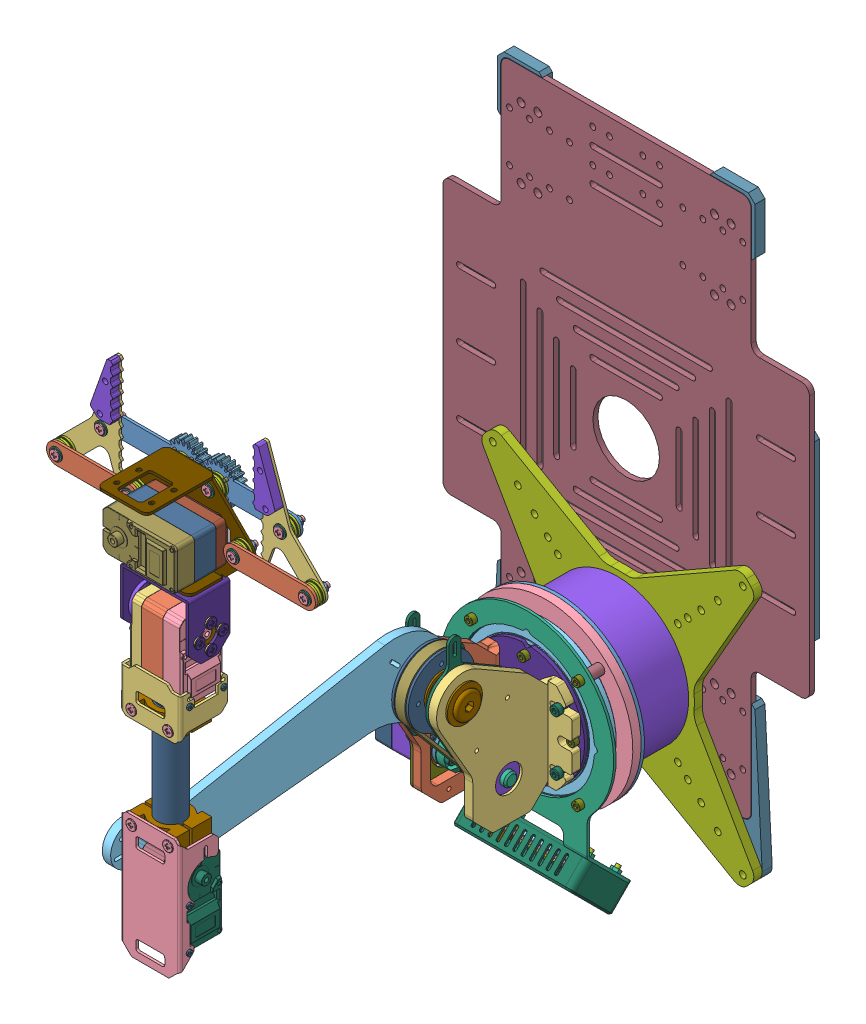
SolidWorks assembly RoArm-M1 STEP, configuration Default. Lengths in mm. (continued)
Components (placement in the parent): (continued)
- RoArm-M1 STEP(2)^RoArm-M1 STEP-1: RoArm-M1 STEP(2)^RoArm-M1 STEP [Default] at origin size (176.32 372.07 316.7) (virtual) (continued)
  - Servo Driver with ESP32^RoArm-M1 STEP(2)_RoArm-M1 STEP-1: Servo Driver with ESP32^RoArm-M1 STEP(2)_RoArm-M1 STEP [Default] at (-32.5 -89.0448 39.0323) x (1 0 0) z (0 -0.707107 0.707107) size (65.89 30.51 11.2) (virtual) (continued)
    - Servo Driver with ESP32-0^Servo Driver with ESP32_RoArm-M1 STEP(2)_RoArm-M1 STEP-1: Servo Driver with ESP32-0^Servo Driver with ESP32_RoArm-M1 STEP(2)_RoArm-M1 STEP [Default] at origin size (11 5 5.7) (virtual)
    - Servo Driver with ESP32-1^Servo Driver with ESP32_RoArm-M1 STEP(2)_RoArm-M1 STEP-1: Servo Driver with ESP32-1^Servo Driver with ESP32_RoArm-M1 STEP(2)_RoArm-M1 STEP [Default] at origin size (0.71 0.71 7.5) (virtual)
    - Servo Driver with ESP32-2^Servo Driver with ESP32_RoArm-M1 STEP(2)_RoArm-M1 STEP-1: Servo Driver with ESP32-2^Servo Driver with ESP32_RoArm-M1 STEP(2)_RoArm-M1 STEP [Default] at origin size (0.71 0.71 7.5) (virtual)
    - Servo Driver with ESP32-3^Servo Driver with ESP32_RoArm-M1 STEP(2)_RoArm-M1 STEP-1: Servo Driver with ESP32-3^Servo Driver with ESP32_RoArm-M1 STEP(2)_RoArm-M1 STEP [Default] at origin size (0.71 0.71 7.5) (virtual)
    - Servo Driver with ESP32-4^Servo Driver with ESP32_RoArm-M1 STEP(2)_RoArm-M1 STEP-1: Servo Driver with ESP32-4^Servo Driver with ESP32_RoArm-M1 STEP(2)_RoArm-M1 STEP [Default] at origin size (11 5 8.5) (virtual)
    - Servo Driver with ESP32-5^Servo Driver with ESP32_RoArm-M1 STEP(2)_RoArm-M1 STEP-1: Servo Driver with ESP32-5^Servo Driver with ESP32_RoArm-M1 STEP(2)_RoArm-M1 STEP [Default] at origin size (0.7 0.7 7.5) (virtual)
    - Servo Driver with ESP32-6^Servo Driver with ESP32_RoArm-M1 STEP(2)_RoArm-M1 STEP-1: Servo Driver with ESP32-6^Servo Driver with ESP32_RoArm-M1 STEP(2)_RoArm-M1 STEP [Default] at origin size (0.71 0.71 7.5) (virtual)
  - 碳管前固定^RoArm-M1 STEP(2)_RoArm-M1 STEP-1: 碳管前固定^RoArm-M1 STEP(2)_RoArm-M1 STEP [Default] at (66.1341 -832.2469 298.6056) x (0 -1 0) z (0 0 1) size (28.35 36.11 28.3) (virtual)
  - 碳管后固定^RoArm-M1 STEP(2)_RoArm-M1 STEP-1: 碳管后固定^RoArm-M1 STEP(2)_RoArm-M1 STEP [Default] at (-73.8484 -939.3227 298.6056) x (0 -1 0) z (0 0 1) size (73.69 35.71 23.05) (virtual)
  - 机械臂大臂^RoArm-M1 STEP(2)_RoArm-M1 STEP-1: 机械臂大臂^RoArm-M1 STEP(2)_RoArm-M1 STEP [Default] at (-4.9615 -12.5543 693.461) x (0 0 1) z (-1 0 0) size (207.69 52.86 5) (virtual)
  - 中心外侧PCB支架^RoArm-M1 STEP(2)_RoArm-M1 STEP-1: 中心外侧PCB支架^RoArm-M1 STEP(2)_RoArm-M1 STEP [Default] at (18.4653 1675.6917 58) x (0 -1 0) z (0 0 1) size (138.15 104 27.96) (virtual)
  - X型底座^RoArm-M1 STEP(2)_RoArm-M1 STEP-1: X型底座^RoArm-M1 STEP(2)_RoArm-M1 STEP [Default] at (2038.816 -62.8687 0) x (-1 0 0) z (0 0 1) size (163.25 163.25 5) (virtual)
  - 厚铝管^RoArm-M1 STEP(2)_RoArm-M1 STEP-1: 厚铝管^RoArm-M1 STEP(2)_RoArm-M1 STEP [Default] at (0 0 5) x (-1 0 0) z (0 0 1) size (85 85 36) (virtual)
  - LEG-HOLDER^RoArm-M1 STEP(2)_RoArm-M1 STEP-1: LEG-HOLDER^RoArm-M1 STEP(2)_RoArm-M1 STEP [Default] at (14.5485 57.813 287.8556) x (-1 0 0) z (0 1 0) size (28 21.5 10.1) (virtual)
  - LEG-HOLDER^RoArm-M1 STEP(2)_RoArm-M1 STEP-2: LEG-HOLDER^RoArm-M1 STEP(2)_RoArm-M1 STEP [Default] at (14.5485 117.713 287.8556) x (-1 0 0) z (0 1 0) size (28 21.5 10.1) (virtual)
  - 70mm碳纤维管材^RoArm-M1 STEP(2)_RoArm-M1 STEP-1: 70mm碳纤维管材^RoArm-M1 STEP(2)_RoArm-M1 STEP [Default] at (-267.2094 57.813 273.529) x (-1 0 0) z (0 1 0) size (16 16 70) (virtual)
  - 圆形隔离柱 M3_35^RoArm-M1 STEP(2)_RoArm-M1 STEP-1: 圆形隔离柱 M3_35^RoArm-M1 STEP(2)_RoArm-M1 STEP [Default] at (-24.3952 24.3952 5) x (-1 0 0) z (0 0 1) size (6 6 35) (virtual)
  - 圆形隔离柱 M3_35^RoArm-M1 STEP(2)_RoArm-M1 STEP-2: 圆形隔离柱 M3_35^RoArm-M1 STEP(2)_RoArm-M1 STEP [Default] at (-24.3952 -24.3952 5) x (-1 0 0) z (0 0 1) size (6 6 35) (virtual)
  - 圆形隔离柱 M3_35^RoArm-M1 STEP(2)_RoArm-M1 STEP-3: 圆形隔离柱 M3_35^RoArm-M1 STEP(2)_RoArm-M1 STEP [Default] at (24.3952 -24.3952 5) x (-1 0 0) z (0 0 1) size (6 6 35) (virtual)
  - 圆形隔离柱 M3_35^RoArm-M1 STEP(2)_RoArm-M1 STEP-4: 圆形隔离柱 M3_35^RoArm-M1 STEP(2)_RoArm-M1 STEP [Default] at (24.3952 24.3952 5) x (-1 0 0) z (0 0 1) size (6 6 35) (virtual)
  - 黑色金属沉头螺丝 KM3_10^RoArm-M1 STEP(2)_RoArm-M1 STEP-1: 黑色金属沉头螺丝 KM3_10^RoArm-M1 STEP(2)_RoArm-M1 STEP [Default] at (24.3952 -24.3952 12) x (-1 0 0) z (0 0 -1) size (5.2 5.2 6) (virtual)
  - 黑色金属沉头螺丝 KM3_10^RoArm-M1 STEP(2)_RoArm-M1 STEP-2: 黑色金属沉头螺丝 KM3_10^RoArm-M1 STEP(2)_RoArm-M1 STEP [Default] at (24.3952 24.3952 12) x (-1 0 0) z (0 0 -1) size (5.2 5.2 6) (virtual)
  - 黑色金属沉头螺丝 KM3_10^RoArm-M1 STEP(2)_RoArm-M1 STEP-3: 黑色金属沉头螺丝 KM3_10^RoArm-M1 STEP(2)_RoArm-M1 STEP [Default] at (-24.3952 -24.3952 12) x (-1 0 0) z (0 0 -1) size (5.2 5.2 6) (virtual)
  - 黑色金属沉头螺丝 KM3_10^RoArm-M1 STEP(2)_RoArm-M1 STEP-4: 黑色金属沉头螺丝 KM3_10^RoArm-M1 STEP(2)_RoArm-M1 STEP [Default] at (-24.3952 24.3952 12) x (-1 0 0) z (0 0 -1) size (5.2 5.2 6) (virtual)
  - 圆形隔离柱 M3_10^RoArm-M1 STEP(2)_RoArm-M1 STEP-1: 圆形隔离柱 M3_10^RoArm-M1 STEP(2)_RoArm-M1 STEP [Default] at (32.1734 -32.1734 48) x (-1 0 0) z (0 0 1) size (6 6 10) (virtual)
  - 圆形隔离柱 M3_10^RoArm-M1 STEP(2)_RoArm-M1 STEP-2: 圆形隔离柱 M3_10^RoArm-M1 STEP(2)_RoArm-M1 STEP [Default] at (32.1734 32.1734 48) x (-1 0 0) z (0 0 1) size (6 6 10) (virtual)
  - 圆形隔离柱 M3_10^RoArm-M1 STEP(2)_RoArm-M1 STEP-3: 圆形隔离柱 M3_10^RoArm-M1 STEP(2)_RoArm-M1 STEP [Default] at (-32.1734 32.1734 48) x (-1 0 0) z (0 0 1) size (6 6 10) (virtual)
  - 圆形隔离柱 M3_10^RoArm-M1 STEP(2)_RoArm-M1 STEP-4: 圆形隔离柱 M3_10^RoArm-M1 STEP(2)_RoArm-M1 STEP [Default] at (-32.1734 -32.1734 48) x (-1 0 0) z (0 0 1) size (6 6 10) (virtual)
  - 黑色金属圆头尖尾自攻螺丝 PA2_5^RoArm-M1 STEP(2)_RoArm-M1 STEP-1: 黑色金属圆头尖尾自攻螺丝 PA2_5^RoArm-M1 STEP(2)_RoArm-M1 STEP [Default] at (8.3 -10.25 43) x (-1 0 0) z (0 0 1) size (3.35 3.35 6.15) (virtual)
  - 黑色金属圆头尖尾自攻螺丝 PA2_5^RoArm-M1 STEP(2)_RoArm-M1 STEP-2: 黑色金属圆头尖尾自攻螺丝 PA2_5^RoArm-M1 STEP(2)_RoArm-M1 STEP [Default] at (29 -10.25 43) x (-1 0 0) z (0 0 1) size (3.35 3.35 6.15) (virtual)
  - 黑色金属圆头尖尾自攻螺丝 PA2_5^RoArm-M1 STEP(2)_RoArm-M1 STEP-3: 黑色金属圆头尖尾自攻螺丝 PA2_5^RoArm-M1 STEP(2)_RoArm-M1 STEP [Default] at (8.3 10.25 43) x (-1 0 0) z (0 0 1) size (3.35 3.35 6.15) (virtual)
  - 黑色金属圆头尖尾自攻螺丝 PA2_5^RoArm-M1 STEP(2)_RoArm-M1 STEP-4: 黑色金属圆头尖尾自攻螺丝 PA2_5^RoArm-M1 STEP(2)_RoArm-M1 STEP [Default] at (29 10.25 43) x (-1 0 0) z (0 0 1) size (3.35 3.35 6.15) (virtual)
  - 黑色金属圆头尖尾自攻螺丝 PA2_5^RoArm-M1 STEP(2)_RoArm-M1 STEP-5: 黑色金属圆头尖尾自攻螺丝 PA2_5^RoArm-M1 STEP(2)_RoArm-M1 STEP [Default] at (-17.9615 -3.5824 98.625) x (0 0 1) z (1 0 0) size (3.35 3.35 6.15) (virtual)
  - 黑色金属圆头尖尾自攻螺丝 PA2_5^RoArm-M1 STEP(2)_RoArm-M1 STEP-6: 黑色金属圆头尖尾自攻螺丝 PA2_5^RoArm-M1 STEP(2)_RoArm-M1 STEP [Default] at (-17.9615 17.1176 98.625) x (0 0 1) z (1 0 0) size (3.35 3.35 6.15) (virtual)
  - 黑色金属圆头尖尾自攻螺丝 PA2_5^RoArm-M1 STEP(2)_RoArm-M1 STEP-7: 黑色金属圆头尖尾自攻螺丝 PA2_5^RoArm-M1 STEP(2)_RoArm-M1 STEP [Default] at (-17.9615 17.1176 78.125) x (0 0 1) z (1 0 0) size (3.35 3.35 6.15) (virtual)
  - 黑色金属圆头尖尾自攻螺丝 PA2_5^RoArm-M1 STEP(2)_RoArm-M1 STEP-8: 黑色金属圆头尖尾自攻螺丝 PA2_5^RoArm-M1 STEP(2)_RoArm-M1 STEP [Default] at (-17.9615 -3.5824 78.125) x (0 0 1) z (1 0 0) size (3.35 3.35 6.15) (virtual)
  - 黑色金属圆头尖尾自攻螺丝 PA2_5^RoArm-M1 STEP(2)_RoArm-M1 STEP-9: 黑色金属圆头尖尾自攻螺丝 PA2_5^RoArm-M1 STEP(2)_RoArm-M1 STEP [Default] at (32.3585 32.7513 294.848) x (0 0 1) z (1 0 0) size (3.35 3.35 6.15) (virtual)
  - 黑色金属圆头尖尾自攻螺丝 PA2_5^RoArm-M1 STEP(2)_RoArm-M1 STEP-10: 黑色金属圆头尖尾自攻螺丝 PA2_5^RoArm-M1 STEP(2)_RoArm-M1 STEP [Default] at (32.3585 8.3013 294.848) x (0 0 1) z (1 0 0) size (3.35 3.35 6.15) (virtual)
  - 黑色金属圆头尖尾自攻螺丝 PA2_5^RoArm-M1 STEP(2)_RoArm-M1 STEP-11: 黑色金属圆头尖尾自攻螺丝 PA2_5^RoArm-M1 STEP(2)_RoArm-M1 STEP [Default] at (-1.7615 12.0513 294.848) x (0 0 -1) z (-1 0 0) size (3.35 3.35 6.15) (virtual)
  - 黑色金属圆头尖尾自攻螺丝 PA2_5^RoArm-M1 STEP(2)_RoArm-M1 STEP-12: 黑色金属圆头尖尾自攻螺丝 PA2_5^RoArm-M1 STEP(2)_RoArm-M1 STEP [Default] at (-1.7615 32.7513 294.848) x (0 0 -1) z (-1 0 0) size (3.35 3.35 6.15) (virtual)
  - 黑色金属圆头尖尾自攻螺丝 PA2_5^RoArm-M1 STEP(2)_RoArm-M1 STEP-13: 黑色金属圆头尖尾自攻螺丝 PA2_5^RoArm-M1 STEP(2)_RoArm-M1 STEP [Default] at (-3.4615 139.9747 294.848) x (0 0 -1) z (-1 0 0) size (3.35 3.35 6.15) (virtual)
  - 黑色金属圆头尖尾自攻螺丝 PA2_5^RoArm-M1 STEP(2)_RoArm-M1 STEP-14: 黑色金属圆头尖尾自攻螺丝 PA2_5^RoArm-M1 STEP(2)_RoArm-M1 STEP [Default] at (-3.4615 139.9747 274.348) x (0 0 -1) z (-1 0 0) size (3.35 3.35 6.15) (virtual)
  - 黑色金属圆头尖尾自攻螺丝 PA2_5^RoArm-M1 STEP(2)_RoArm-M1 STEP-15: 黑色金属圆头尖尾自攻螺丝 PA2_5^RoArm-M1 STEP(2)_RoArm-M1 STEP [Default] at (32.5585 136.2247 294.848) x (0 0 1) z (1 0 0) size (3.35 3.35 6.15) (virtual)
  - 黑色金属圆头尖尾自攻螺丝 PA2_5^RoArm-M1 STEP(2)_RoArm-M1 STEP-16: 黑色金属圆头尖尾自攻螺丝 PA2_5^RoArm-M1 STEP(2)_RoArm-M1 STEP [Default] at (32.5585 136.2247 274.348) x (0 0 1) z (1 0 0) size (3.35 3.35 6.15) (virtual)
  - 黑色金属圆头尖尾自攻螺丝 PA2_5^RoArm-M1 STEP(2)_RoArm-M1 STEP-17: 黑色金属圆头尖尾自攻螺丝 PA2_5^RoArm-M1 STEP(2)_RoArm-M1 STEP [Default] at (30.4885 203.7559 273.6404) x (0 1 0) z (0 0 -1) size (3.35 3.35 6.15) (virtual)
  - 黑色金属圆头尖尾自攻螺丝 PA2_5^RoArm-M1 STEP(2)_RoArm-M1 STEP-18: 黑色金属圆头尖尾自攻螺丝 PA2_5^RoArm-M1 STEP(2)_RoArm-M1 STEP [Default] at (9.7885 203.7559 273.6404) x (0 1 0) z (0 0 -1) size (3.35 3.35 6.15) (virtual)
  - 黑色金属圆头尖尾自攻螺丝 PA2_5^RoArm-M1 STEP(2)_RoArm-M1 STEP-19: 黑色金属圆头尖尾自攻螺丝 PA2_5^RoArm-M1 STEP(2)_RoArm-M1 STEP [Default] at (30.4885 224.2559 273.6404) x (0 1 0) z (0 0 -1) size (3.35 3.35 6.15) (virtual)
  - 黑色金属圆头尖尾自攻螺丝 PA2_5^RoArm-M1 STEP(2)_RoArm-M1 STEP-20: 黑色金属圆头尖尾自攻螺丝 PA2_5^RoArm-M1 STEP(2)_RoArm-M1 STEP [Default] at (9.7885 224.2559 273.6404) x (0 1 0) z (0 0 -1) size (3.35 3.35 6.15) (virtual)
  - 黑色金属杯头内六角螺丝 M3_8^RoArm-M1 STEP(2)_RoArm-M1 STEP-1: 黑色金属杯头内六角螺丝 M3_8^RoArm-M1 STEP(2)_RoArm-M1 STEP [Default] at (-11.2615 -11.8824 95.375) x (0 0 1) z (1 0 0) size (5.5 5.5 11.1) (virtual)
  - 黑色金属杯头内六角螺丝 M3_8^RoArm-M1 STEP(2)_RoArm-M1 STEP-2: 黑色金属杯头内六角螺丝 M3_8^RoArm-M1 STEP(2)_RoArm-M1 STEP [Default] at (-16.2615 -11.8824 88.375) x (0 0 1) z (1 0 0) size (5.5 5.5 11.1) (virtual)
  - 黑色金属杯头内六角螺丝 M3_8^RoArm-M1 STEP(2)_RoArm-M1 STEP-3: 黑色金属杯头内六角螺丝 M3_8^RoArm-M1 STEP(2)_RoArm-M1 STEP [Default] at (-11.2615 -18.8824 88.375) x (0 0 1) z (1 0 0) size (5.5 5.5 11.1) (virtual)
  - 黑色金属杯头内六角螺丝 M3_8^RoArm-M1 STEP(2)_RoArm-M1 STEP-4: 黑色金属杯头内六角螺丝 M3_8^RoArm-M1 STEP(2)_RoArm-M1 STEP [Default] at (-11.2615 -4.8824 88.375) x (0 0 1) z (1 0 0) size (5.5 5.5 11.1) (virtual)
  - 黑色金属杯头内六角螺丝 M3_8^RoArm-M1 STEP(2)_RoArm-M1 STEP-5: 黑色金属杯头内六角螺丝 M3_8^RoArm-M1 STEP(2)_RoArm-M1 STEP [Default] at (-11.2615 -11.8824 81.375) x (0 0 1) z (1 0 0) size (5.5 5.5 11.1) (virtual)
  - 黑色金属杯头内六角螺丝 M3_8^RoArm-M1 STEP(2)_RoArm-M1 STEP-6: 黑色金属杯头内六角螺丝 M3_8^RoArm-M1 STEP(2)_RoArm-M1 STEP [Default] at (24.9 -16.5003 65) x (-1 0 0) z (0 0 1) size (5.5 5.5 11.1) (virtual)
  - 黑色金属杯头内六角螺丝 M3_8^RoArm-M1 STEP(2)_RoArm-M1 STEP-7: 黑色金属杯头内六角螺丝 M3_8^RoArm-M1 STEP(2)_RoArm-M1 STEP [Default] at (24.9 16.5003 65) x (-1 0 0) z (0 0 1) size (5.5 5.5 11.1) (virtual)
  - 黑色金属杯头内六角螺丝 M3_8^RoArm-M1 STEP(2)_RoArm-M1 STEP-8: 黑色金属杯头内六角螺丝 M3_8^RoArm-M1 STEP(2)_RoArm-M1 STEP [Default] at (-24.9 -16.5003 65) x (-1 0 0) z (0 0 1) size (5.5 5.5 11.1) (virtual)
  - 黑色金属杯头内六角螺丝 M3_8^RoArm-M1 STEP(2)_RoArm-M1 STEP-9: 黑色金属杯头内六角螺丝 M3_8^RoArm-M1 STEP(2)_RoArm-M1 STEP [Default] at (-24.9 16.5003 65) x (-1 0 0) z (0 0 1) size (5.5 5.5 11.1) (virtual)
  - 银色金属杯头内六角螺丝 M3_6^RoArm-M1 STEP(2)_RoArm-M1 STEP-1: 银色金属杯头内六角螺丝 M3_6^RoArm-M1 STEP(2)_RoArm-M1 STEP [Default] at (-32.1734 32.1734 59.5) x (-1 0 0) z (0 0 1) size (5 5 9.1) (virtual)
  - 银色金属杯头内六角螺丝 M3_6^RoArm-M1 STEP(2)_RoArm-M1 STEP-2: 银色金属杯头内六角螺丝 M3_6^RoArm-M1 STEP(2)_RoArm-M1 STEP [Default] at (-32.1734 -32.1734 59.5) x (-1 0 0) z (0 0 1) size (5 5 9.1) (virtual)
  - 银色金属杯头内六角螺丝 M3_6^RoArm-M1 STEP(2)_RoArm-M1 STEP-3: 银色金属杯头内六角螺丝 M3_6^RoArm-M1 STEP(2)_RoArm-M1 STEP [Default] at (32.1734 32.1734 59.5) x (-1 0 0) z (0 0 1) size (5 5 9.1) (virtual)
  - 银色金属杯头内六角螺丝 M3_6^RoArm-M1 STEP(2)_RoArm-M1 STEP-4: 银色金属杯头内六角螺丝 M3_6^RoArm-M1 STEP(2)_RoArm-M1 STEP [Default] at (32.1734 -32.1734 59.5) x (-1 0 0) z (0 0 1) size (5 5 9.1) (virtual)
  - 圆形隔离柱 M3_10^RoArm-M1 STEP(2)_RoArm-M1 STEP-5: 圆形隔离柱 M3_10^RoArm-M1 STEP(2)_RoArm-M1 STEP [Default] at (29.5 0 48) x (-1 0 0) z (0 0 1) size (6 6 10) (virtual)
  - 圆形隔离柱 M3_10^RoArm-M1 STEP(2)_RoArm-M1 STEP-6: 圆形隔离柱 M3_10^RoArm-M1 STEP(2)_RoArm-M1 STEP [Default] at (0 29.5 48) x (-1 0 0) z (0 0 1) size (6 6 10) (virtual)
  - 圆形隔离柱 M3_10^RoArm-M1 STEP(2)_RoArm-M1 STEP-7: 圆形隔离柱 M3_10^RoArm-M1 STEP(2)_RoArm-M1 STEP [Default] at (-29.5 0 48) x (-1 0 0) z (0 0 1) size (6 6 10) (virtual)
  - 圆形隔离柱 M3_10^RoArm-M1 STEP(2)_RoArm-M1 STEP-8: 圆形隔离柱 M3_10^RoArm-M1 STEP(2)_RoArm-M1 STEP [Default] at (0 -29.5 48) x (-1 0 0) z (0 0 1) size (6 6 10) (virtual)
  - 银色金属杯头内六角螺丝 M3_6^RoArm-M1 STEP(2)_RoArm-M1 STEP-5: 银色金属杯头内六角螺丝 M3_6^RoArm-M1 STEP(2)_RoArm-M1 STEP [Default] at (29.5 0 60) x (-1 0 0) z (0 0 1) size (5 5 9.1) (virtual)
  - 银色金属杯头内六角螺丝 M3_6^RoArm-M1 STEP(2)_RoArm-M1 STEP-6: 银色金属杯头内六角螺丝 M3_6^RoArm-M1 STEP(2)_RoArm-M1 STEP [Default] at (0 29.5 60) x (-1 0 0) z (0 0 1) size (5 5 9.1) (virtual)
  - 银色金属杯头内六角螺丝 M3_6^RoArm-M1 STEP(2)_RoArm-M1 STEP-7: 银色金属杯头内六角螺丝 M3_6^RoArm-M1 STEP(2)_RoArm-M1 STEP [Default] at (-29.5 0 60) x (-1 0 0) z (0 0 1) size (5 5 9.1) (virtual)
  - 银色金属杯头内六角螺丝 M3_6^RoArm-M1 STEP(2)_RoArm-M1 STEP-8: 银色金属杯头内六角螺丝 M3_6^RoArm-M1 STEP(2)_RoArm-M1 STEP [Default] at (0 -29.5 60) x (-1 0 0) z (0 0 1) size (5 5 9.1) (virtual)
  - 黑色金属扁平头螺丝 CM3_6_6^RoArm-M1 STEP(2)_RoArm-M1 STEP-1: 黑色金属扁平头螺丝 CM3_6_6^RoArm-M1 STEP(2)_RoArm-M1 STEP [Default] at (24.3952 24.3952 43) x (-1 0 0) z (0 0 1) size (6 6 6.8) (virtual)
  - 黑色金属扁平头螺丝 CM3_6_6^RoArm-M1 STEP(2)_RoArm-M1 STEP-2: 黑色金属扁平头螺丝 CM3_6_6^RoArm-M1 STEP(2)_RoArm-M1 STEP [Default] at (-24.3952 24.3952 43) x (-1 0 0) z (0 0 1) size (6 6 6.8) (virtual)
  - 黑色金属扁平头螺丝 CM3_6_6^RoArm-M1 STEP(2)_RoArm-M1 STEP-3: 黑色金属扁平头螺丝 CM3_6_6^RoArm-M1 STEP(2)_RoArm-M1 STEP [Default] at (24.3952 -24.3952 43) x (-1 0 0) z (0 0 1) size (6 6 6.8) (virtual)
  - 黑色金属扁平头螺丝 CM3_6_6^RoArm-M1 STEP(2)_RoArm-M1 STEP-4: 黑色金属扁平头螺丝 CM3_6_6^RoArm-M1 STEP(2)_RoArm-M1 STEP [Default] at (-24.3952 -24.3952 43) x (-1 0 0) z (0 0 1) size (6 6 6.8) (virtual)
  - 黑色金属扁平头螺丝 CM3_6_6^RoArm-M1 STEP(2)_RoArm-M1 STEP-5: 黑色金属扁平头螺丝 CM3_6_6^RoArm-M1 STEP(2)_RoArm-M1 STEP [Default] at (29.5 0 46) x (-1 0 0) z (0 0 -1) size (6 6 6.8) (virtual)
  - 黑色金属扁平头螺丝 CM3_6_6^RoArm-M1 STEP(2)_RoArm-M1 STEP-6: 黑色金属扁平头螺丝 CM3_6_6^RoArm-M1 STEP(2)_RoArm-M1 STEP [Default] at (0 29.5 46) x (-1 0 0) z (0 0 -1) size (6 6 6.8) (virtual)
  - 黑色金属扁平头螺丝 CM3_6_6^RoArm-M1 STEP(2)_RoArm-M1 STEP-7: 黑色金属扁平头螺丝 CM3_6_6^RoArm-M1 STEP(2)_RoArm-M1 STEP [Default] at (0 -29.5 46) x (-1 0 0) z (0 0 -1) size (6 6 6.8) (virtual)
  - 黑色金属扁平头螺丝 CM3_6_6^RoArm-M1 STEP(2)_RoArm-M1 STEP-8: 黑色金属扁平头螺丝 CM3_6_6^RoArm-M1 STEP(2)_RoArm-M1 STEP [Default] at (-29.5 0 46) x (-1 0 0) z (0 0 -1) size (6 6 6.8) (virtual)
  - 黑色金属扁平头螺丝 CM3_6_6^RoArm-M1 STEP(2)_RoArm-M1 STEP-9: 黑色金属扁平头螺丝 CM3_6_6^RoArm-M1 STEP(2)_RoArm-M1 STEP [Default] at (0 0 45.2) x (-1 0 0) z (0 0 1) size (6 6 6.8) (virtual)
  - 黑色金属扁平头螺丝 CM3_6_6^RoArm-M1 STEP(2)_RoArm-M1 STEP-10: 黑色金属扁平头螺丝 CM3_6_6^RoArm-M1 STEP(2)_RoArm-M1 STEP [Default] at (-7 0 49) x (-1 0 0) z (0 0 1) size (6 6 6.8) (virtual)
  - 黑色金属扁平头螺丝 CM3_6_6^RoArm-M1 STEP(2)_RoArm-M1 STEP-11: 黑色金属扁平头螺丝 CM3_6_6^RoArm-M1 STEP(2)_RoArm-M1 STEP [Default] at (0 -7 49) x (-1 0 0) z (0 0 1) size (6 6 6.8) (virtual)
  - 黑色金属扁平头螺丝 CM3_6_6^RoArm-M1 STEP(2)_RoArm-M1 STEP-12: 黑色金属扁平头螺丝 CM3_6_6^RoArm-M1 STEP(2)_RoArm-M1 STEP [Default] at (7 0 49) x (-1 0 0) z (0 0 1) size (6 6 6.8) (virtual)
  - 黑色金属扁平头螺丝 CM3_6_6^RoArm-M1 STEP(2)_RoArm-M1 STEP-13: 黑色金属扁平头螺丝 CM3_6_6^RoArm-M1 STEP(2)_RoArm-M1 STEP [Default] at (0 7 49) x (-1 0 0) z (0 0 1) size (6 6 6.8) (virtual)
  - 黑色金属杯头内六角螺丝 M3_10^RoArm-M1 STEP(2)_RoArm-M1 STEP-1: 黑色金属杯头内六角螺丝 M3_10^RoArm-M1 STEP(2)_RoArm-M1 STEP [Default] at (-32.1734 32.1734 41) x (1 0 0) z (0 0 -1) size (5 5 13.1) (virtual)
  - 黑色金属杯头内六角螺丝 M3_10^RoArm-M1 STEP(2)_RoArm-M1 STEP-2: 黑色金属杯头内六角螺丝 M3_10^RoArm-M1 STEP(2)_RoArm-M1 STEP [Default] at (-32.1734 -32.1734 41) x (1 0 0) z (0 0 -1) size (5 5 13.1) (virtual)
  - 黑色金属杯头内六角螺丝 M3_10^RoArm-M1 STEP(2)_RoArm-M1 STEP-3: 黑色金属杯头内六角螺丝 M3_10^RoArm-M1 STEP(2)_RoArm-M1 STEP [Default] at (32.1734 -32.1734 41) x (1 0 0) z (0 0 -1) size (5 5 13.1) (virtual)
  - 黑色金属杯头内六角螺丝 M3_10^RoArm-M1 STEP(2)_RoArm-M1 STEP-4: 黑色金属杯头内六角螺丝 M3_10^RoArm-M1 STEP(2)_RoArm-M1 STEP [Default] at (32.1734 32.1734 41) x (1 0 0) z (0 0 -1) size (5 5 13.1) (virtual)
  - 银色金属扁平头螺丝 CM3_4_6^RoArm-M1 STEP(2)_RoArm-M1 STEP-1: 银色金属扁平头螺丝 CM3_4_6^RoArm-M1 STEP(2)_RoArm-M1 STEP [Default] at (-19.4615 12.2829 107.6065) x (0 0 -1) z (-1 0 0) size (6 6 4.8) (virtual)
  - 银色金属扁平头螺丝 CM3_4_6^RoArm-M1 STEP(2)_RoArm-M1 STEP-2: 银色金属扁平头螺丝 CM3_4_6^RoArm-M1 STEP(2)_RoArm-M1 STEP [Default] at (-11.4615 12.2829 107.6065) x (0 0 -1) z (1 0 0) size (6 6 4.8) (virtual)
  - 银色金属扁平头螺丝 CM3_4_6^RoArm-M1 STEP(2)_RoArm-M1 STEP-3: 银色金属扁平头螺丝 CM3_4_6^RoArm-M1 STEP(2)_RoArm-M1 STEP [Default] at (-11.4615 30.6677 89.2217) x (0 0 -1) z (1 0 0) size (6 6 4.8) (virtual)
  - 银色金属扁平头螺丝 CM3_4_6^RoArm-M1 STEP(2)_RoArm-M1 STEP-4: 银色金属扁平头螺丝 CM3_4_6^RoArm-M1 STEP(2)_RoArm-M1 STEP [Default] at (-19.4615 30.6677 89.2217) x (0 0 -1) z (-1 0 0) size (6 6 4.8) (virtual)
  - 银色金属扁平头螺丝 CM3_4_6^RoArm-M1 STEP(2)_RoArm-M1 STEP-5: 银色金属扁平头螺丝 CM3_4_6^RoArm-M1 STEP(2)_RoArm-M1 STEP [Default] at (-19.4615 -30.1733 93.375) x (0 0 -1) z (-1 0 0) size (6 6 4.8) (virtual)
  - 银色金属扁平头螺丝 CM3_4_6^RoArm-M1 STEP(2)_RoArm-M1 STEP-6: 银色金属扁平头螺丝 CM3_4_6^RoArm-M1 STEP(2)_RoArm-M1 STEP [Default] at (-19.4615 -30.1733 81.375) x (0 0 -1) z (-1 0 0) size (6 6 4.8) (virtual)
  - 银色金属扁平头螺丝 CM3_4_6^RoArm-M1 STEP(2)_RoArm-M1 STEP-7: 银色金属扁平头螺丝 CM3_4_6^RoArm-M1 STEP(2)_RoArm-M1 STEP [Default] at (11.4615 30.6677 89.2217) x (0 0 -1) z (-1 0 0) size (6 6 4.8) (virtual)
  - 银色金属扁平头螺丝 CM3_4_6^RoArm-M1 STEP(2)_RoArm-M1 STEP-8: 银色金属扁平头螺丝 CM3_4_6^RoArm-M1 STEP(2)_RoArm-M1 STEP [Default] at (11.4615 12.2829 107.6065) x (0 0 -1) z (-1 0 0) size (6 6 4.8) (virtual)
  - 银色金属扁平头螺丝 CM3_10^RoArm-M1 STEP(2)_RoArm-M1 STEP-1: 银色金属扁平头螺丝 CM3_10^RoArm-M1 STEP(2)_RoArm-M1 STEP [Default] at (-9.9615 41.0513 129.7401) x (0 0 -1) z (-1 0 0) size (6 6 11) (virtual)
  - 银色金属扁平头螺丝 CM3_10^RoArm-M1 STEP(2)_RoArm-M1 STEP-2: 银色金属扁平头螺丝 CM3_10^RoArm-M1 STEP(2)_RoArm-M1 STEP [Default] at (-9.9615 27.0513 115.7401) x (0 0 -1) z (-1 0 0) size (6 6 11) (virtual)
  - 银色金属扁平头螺丝 CM3_10^RoArm-M1 STEP(2)_RoArm-M1 STEP-3: 银色金属扁平头螺丝 CM3_10^RoArm-M1 STEP(2)_RoArm-M1 STEP [Default] at (-9.9615 55.0513 115.7401) x (0 0 -1) z (-1 0 0) size (6 6 11) (virtual)
  - 银色金属扁平头螺丝 CM3_10^RoArm-M1 STEP(2)_RoArm-M1 STEP-4: 银色金属扁平头螺丝 CM3_10^RoArm-M1 STEP(2)_RoArm-M1 STEP [Default] at (-9.9615 41.0513 101.7401) x (0 0 -1) z (-1 0 0) size (6 6 11) (virtual)
  - 黑色金属杯头内六角螺丝 M3_10^RoArm-M1 STEP(2)_RoArm-M1 STEP-5: 黑色金属杯头内六角螺丝 M3_10^RoArm-M1 STEP(2)_RoArm-M1 STEP [Default] at (-10.8415 41.0513 284.598) x (0 0 -1) z (-1 0 0) size (5 5 13.1) (virtual)
  - 弹性垫片 M3^RoArm-M1 STEP(2)_RoArm-M1 STEP-1: 弹性垫片 M3^RoArm-M1 STEP(2)_RoArm-M1 STEP [Default] at (-9.9615 48.0513 284.598) x (0 0 -1) z (-1 0 0) size (5.2 5.2 0.88) (virtual)
  - 弹性垫片 M3^RoArm-M1 STEP(2)_RoArm-M1 STEP-2: 弹性垫片 M3^RoArm-M1 STEP(2)_RoArm-M1 STEP [Default] at (-9.9615 41.0513 291.598) x (0 0 -1) z (-1 0 0) size (5.2 5.2 0.88) (virtual)
  - 弹性垫片 M3^RoArm-M1 STEP(2)_RoArm-M1 STEP-3: 弹性垫片 M3^RoArm-M1 STEP(2)_RoArm-M1 STEP [Default] at (-9.9615 41.0513 277.598) x (0 0 -1) z (-1 0 0) size (5.2 5.2 0.88) (virtual)
  - 弹性垫片 M3^RoArm-M1 STEP(2)_RoArm-M1 STEP-4: 弹性垫片 M3^RoArm-M1 STEP(2)_RoArm-M1 STEP [Default] at (-9.9615 34.0513 284.598) x (0 0 -1) z (-1 0 0) size (5.2 5.2 0.88) (virtual)
  - 弹性垫片 M3^RoArm-M1 STEP(2)_RoArm-M1 STEP-5: 弹性垫片 M3^RoArm-M1 STEP(2)_RoArm-M1 STEP [Default] at (-9.9615 41.0513 284.598) x (0 0 -1) z (-1 0 0) size (5.2 5.2 0.88) (virtual)
  - 黑色金属杯头内六角螺丝 M3_10^RoArm-M1 STEP(2)_RoArm-M1 STEP-6: 黑色金属杯头内六角螺丝 M3_10^RoArm-M1 STEP(2)_RoArm-M1 STEP [Default] at (-10.8415 41.0513 277.598) x (0 0 -1) z (-1 0 0) size (5 5 13.1) (virtual)
  - 黑色金属杯头内六角螺丝 M3_10^RoArm-M1 STEP(2)_RoArm-M1 STEP-7: 黑色金属杯头内六角螺丝 M3_10^RoArm-M1 STEP(2)_RoArm-M1 STEP [Default] at (-10.8415 34.0513 284.598) x (0 0 -1) z (-1 0 0) size (5 5 13.1) (virtual)
  - 黑色金属杯头内六角螺丝 M3_10^RoArm-M1 STEP(2)_RoArm-M1 STEP-8: 黑色金属杯头内六角螺丝 M3_10^RoArm-M1 STEP(2)_RoArm-M1 STEP [Default] at (-10.8415 48.0513 284.598) x (0 0 -1) z (-1 0 0) size (5 5 13.1) (virtual)
  - 黑色金属杯头内六角螺丝 M3_10^RoArm-M1 STEP(2)_RoArm-M1 STEP-9: 黑色金属杯头内六角螺丝 M3_10^RoArm-M1 STEP(2)_RoArm-M1 STEP [Default] at (-10.8415 41.0513 291.598) x (0 0 -1) z (-1 0 0) size (5 5 13.1) (virtual)
  - 弹性垫片 M3^RoArm-M1 STEP(2)_RoArm-M1 STEP-6: 弹性垫片 M3^RoArm-M1 STEP(2)_RoArm-M1 STEP [Default] at (-6.5215 175.9747 284.598) x (0 0 -1) z (-1 0 0) size (5.2 5.2 0.88) (virtual)
  - 弹性垫片 M3^RoArm-M1 STEP(2)_RoArm-M1 STEP-7: 弹性垫片 M3^RoArm-M1 STEP(2)_RoArm-M1 STEP [Default] at (-6.5215 168.9747 277.598) x (0 0 -1) z (-1 0 0) size (5.2 5.2 0.88) (virtual)
  - 弹性垫片 M3^RoArm-M1 STEP(2)_RoArm-M1 STEP-8: 弹性垫片 M3^RoArm-M1 STEP(2)_RoArm-M1 STEP [Default] at (-6.5215 161.9747 284.598) x (0 0 -1) z (-1 0 0) size (5.2 5.2 0.88) (virtual)
  - 弹性垫片 M3^RoArm-M1 STEP(2)_RoArm-M1 STEP-9: 弹性垫片 M3^RoArm-M1 STEP(2)_RoArm-M1 STEP [Default] at (-6.5215 168.9747 291.598) x (0 0 -1) z (-1 0 0) size (5.2 5.2 0.88) (virtual)
  - 弹性垫片 M3^RoArm-M1 STEP(2)_RoArm-M1 STEP-10: 弹性垫片 M3^RoArm-M1 STEP(2)_RoArm-M1 STEP [Default] at (-4.6615 168.9747 284.598) x (0 0 -1) z (-1 0 0) size (5.2 5.2 0.88) (virtual)
  - 黑色金属扁平头螺丝 CM3_6_6^RoArm-M1 STEP(2)_RoArm-M1 STEP-14: 黑色金属扁平头螺丝 CM3_6_6^RoArm-M1 STEP(2)_RoArm-M1 STEP [Default] at (-5.5415 168.9747 284.598) x (0 0 1) z (-1 0 0) size (6 6 6.8) (virtual)
  - 黑色金属扁平头螺丝 CM3_6_6^RoArm-M1 STEP(2)_RoArm-M1 STEP-15: 黑色金属扁平头螺丝 CM3_6_6^RoArm-M1 STEP(2)_RoArm-M1 STEP [Default] at (-7.4015 168.9747 291.598) x (0 0 1) z (-1 0 0) size (6 6 6.8) (virtual)
  - 黑色金属扁平头螺丝 CM3_6_6^RoArm-M1 STEP(2)_RoArm-M1 STEP-16: 黑色金属扁平头螺丝 CM3_6_6^RoArm-M1 STEP(2)_RoArm-M1 STEP [Default] at (-7.4015 175.9747 284.598) x (0 0 1) z (-1 0 0) size (6 6 6.8) (virtual)
  - 黑色金属扁平头螺丝 CM3_6_6^RoArm-M1 STEP(2)_RoArm-M1 STEP-17: 黑色金属扁平头螺丝 CM3_6_6^RoArm-M1 STEP(2)_RoArm-M1 STEP [Default] at (-7.4015 168.9747 277.598) x (0 0 1) z (-1 0 0) size (6 6 6.8) (virtual)
  - 黑色金属扁平头螺丝 CM3_6_6^RoArm-M1 STEP(2)_RoArm-M1 STEP-18: 黑色金属扁平头螺丝 CM3_6_6^RoArm-M1 STEP(2)_RoArm-M1 STEP [Default] at (-7.4015 161.9747 284.598) x (0 0 1) z (-1 0 0) size (6 6 6.8) (virtual)
  - 弹性垫片 M3^RoArm-M1 STEP(2)_RoArm-M1 STEP-11: 弹性垫片 M3^RoArm-M1 STEP(2)_RoArm-M1 STEP [Default] at (34.4985 161.9747 284.598) x (0 0 -1) z (1 0 0) size (5.2 5.2 0.88) (virtual)
  - 弹性垫片 M3^RoArm-M1 STEP(2)_RoArm-M1 STEP-12: 弹性垫片 M3^RoArm-M1 STEP(2)_RoArm-M1 STEP [Default] at (34.4985 168.9747 291.598) x (0 0 -1) z (1 0 0) size (5.2 5.2 0.88) (virtual)
  - 弹性垫片 M3^RoArm-M1 STEP(2)_RoArm-M1 STEP-13: 弹性垫片 M3^RoArm-M1 STEP(2)_RoArm-M1 STEP [Default] at (34.4985 175.9747 284.598) x (0 0 -1) z (1 0 0) size (5.2 5.2 0.88) (virtual)
  - 弹性垫片 M3^RoArm-M1 STEP(2)_RoArm-M1 STEP-14: 弹性垫片 M3^RoArm-M1 STEP(2)_RoArm-M1 STEP [Default] at (34.4985 168.9747 277.598) x (0 0 -1) z (1 0 0) size (5.2 5.2 0.88) (virtual)
  - 黑色金属扁平头螺丝 CM3_6_6^RoArm-M1 STEP(2)_RoArm-M1 STEP-19: 黑色金属扁平头螺丝 CM3_6_6^RoArm-M1 STEP(2)_RoArm-M1 STEP [Default] at (35.3785 168.9747 291.598) x (0 0 1) z (1 0 0) size (6 6 6.8) (virtual)
  - 黑色金属扁平头螺丝 CM3_6_6^RoArm-M1 STEP(2)_RoArm-M1 STEP-20: 黑色金属扁平头螺丝 CM3_6_6^RoArm-M1 STEP(2)_RoArm-M1 STEP [Default] at (35.3785 161.9747 284.598) x (0 0 1) z (1 0 0) size (6 6 6.8) (virtual)
  - 黑色金属扁平头螺丝 CM3_6_6^RoArm-M1 STEP(2)_RoArm-M1 STEP-21: 黑色金属扁平头螺丝 CM3_6_6^RoArm-M1 STEP(2)_RoArm-M1 STEP [Default] at (35.3785 168.9747 277.598) x (0 0 1) z (1 0 0) size (6 6 6.8) (virtual)
  - 黑色金属扁平头螺丝 CM3_6_6^RoArm-M1 STEP(2)_RoArm-M1 STEP-22: 黑色金属扁平头螺丝 CM3_6_6^RoArm-M1 STEP(2)_RoArm-M1 STEP [Default] at (35.3785 175.9747 284.598) x (0 0 1) z (1 0 0) size (6 6 6.8) (virtual)
  - 黑色金属扁平头螺丝 CM3_6_6^RoArm-M1 STEP(2)_RoArm-M1 STEP-23: 黑色金属扁平头螺丝 CM3_6_6^RoArm-M1 STEP(2)_RoArm-M1 STEP [Default] at (9.0388 190.0347 289.5477) x (0 0 1) z (0 -1 0) size (6 6 6.8) (virtual)
  - 弹性垫片 M3^RoArm-M1 STEP(2)_RoArm-M1 STEP-15: 弹性垫片 M3^RoArm-M1 STEP(2)_RoArm-M1 STEP [Default] at (9.0388 190.9147 289.5477) x (0 0 -1) z (0 -1 0) size (5.2 5.2 0.88) (virtual)
  - 弹性垫片 M3^RoArm-M1 STEP(2)_RoArm-M1 STEP-16: 弹性垫片 M3^RoArm-M1 STEP(2)_RoArm-M1 STEP [Default] at (18.9383 190.9147 289.5477) x (0 0 -1) z (0 -1 0) size (5.2 5.2 0.88) (virtual)
  - 弹性垫片 M3^RoArm-M1 STEP(2)_RoArm-M1 STEP-17: 弹性垫片 M3^RoArm-M1 STEP(2)_RoArm-M1 STEP [Default] at (9.0388 190.9147 279.6482) x (0 0 -1) z (0 -1 0) size (5.2 5.2 0.88) (virtual)
  - 弹性垫片 M3^RoArm-M1 STEP(2)_RoArm-M1 STEP-18: 弹性垫片 M3^RoArm-M1 STEP(2)_RoArm-M1 STEP [Default] at (18.9383 190.9147 279.6482) x (0 0 -1) z (0 -1 0) size (5.2 5.2 0.88) (virtual)
  - 黑色金属扁平头螺丝 CM3_6_6^RoArm-M1 STEP(2)_RoArm-M1 STEP-24: 黑色金属扁平头螺丝 CM3_6_6^RoArm-M1 STEP(2)_RoArm-M1 STEP [Default] at (9.0388 190.0347 279.6482) x (0 0 1) z (0 -1 0) size (6 6 6.8) (virtual)
  - 黑色金属扁平头螺丝 CM3_6_6^RoArm-M1 STEP(2)_RoArm-M1 STEP-25: 黑色金属扁平头螺丝 CM3_6_6^RoArm-M1 STEP(2)_RoArm-M1 STEP [Default] at (18.9383 190.0347 289.5477) x (0 0 1) z (0 -1 0) size (6 6 6.8) (virtual)
  - 黑色金属扁平头螺丝 CM3_6_6^RoArm-M1 STEP(2)_RoArm-M1 STEP-26: 黑色金属扁平头螺丝 CM3_6_6^RoArm-M1 STEP(2)_RoArm-M1 STEP [Default] at (18.9383 190.0347 279.6482) x (0 0 1) z (0 -1 0) size (6 6 6.8) (virtual)
  - 黑色金属扁平头螺丝 CM3_14_6^RoArm-M1 STEP(2)_RoArm-M1 STEP-1: 黑色金属扁平头螺丝 CM3_14_6^RoArm-M1 STEP(2)_RoArm-M1 STEP [Default] at (45.4885 213.9105 281.7404) x (-1 0 0) z (0 0 1) size (6 6 14.8) (virtual)
  - 黑色金属扁平头螺丝 CM3_14_6^RoArm-M1 STEP(2)_RoArm-M1 STEP-2: 黑色金属扁平头螺丝 CM3_14_6^RoArm-M1 STEP(2)_RoArm-M1 STEP [Default] at (88.6885 213.9105 281.7404) x (-1 0 0) z (0 0 1) size (6 6 14.8) (virtual)
  - 黑色金属扁平头螺丝 CM3_14_6^RoArm-M1 STEP(2)_RoArm-M1 STEP-3: 黑色金属扁平头螺丝 CM3_14_6^RoArm-M1 STEP(2)_RoArm-M1 STEP [Default] at (24.4885 234.9105 275.7404) x (-1 0 0) z (0 0 1) size (6 6 14.8) (virtual)
  - 黑色金属扁平头螺丝 CM3_14_6^RoArm-M1 STEP(2)_RoArm-M1 STEP-4: 黑色金属扁平头螺丝 CM3_14_6^RoArm-M1 STEP(2)_RoArm-M1 STEP [Default] at (67.6885 234.9105 275.7404) x (-1 0 0) z (0 0 1) size (6 6 14.8) (virtual)
  - 黑色金属扁平头螺丝 CM3_14_6^RoArm-M1 STEP(2)_RoArm-M1 STEP-5: 黑色金属扁平头螺丝 CM3_14_6^RoArm-M1 STEP(2)_RoArm-M1 STEP [Default] at (3.4885 234.9105 275.7404) x (-1 0 0) z (0 0 1) size (6 6 14.8) (virtual)
  - 黑色金属扁平头螺丝 CM3_14_6^RoArm-M1 STEP(2)_RoArm-M1 STEP-6: 黑色金属扁平头螺丝 CM3_14_6^RoArm-M1 STEP(2)_RoArm-M1 STEP [Default] at (-39.7115 234.9105 275.7404) x (-1 0 0) z (0 0 1) size (6 6 14.8) (virtual)
  - 黑色金属扁平头螺丝 CM3_14_6^RoArm-M1 STEP(2)_RoArm-M1 STEP-7: 黑色金属扁平头螺丝 CM3_14_6^RoArm-M1 STEP(2)_RoArm-M1 STEP [Default] at (-17.5115 213.9105 281.7404) x (-1 0 0) z (0 0 1) size (6 6 14.8) (virtual)
  - 黑色金属扁平头螺丝 CM3_14_6^RoArm-M1 STEP(2)_RoArm-M1 STEP-8: 黑色金属扁平头螺丝 CM3_14_6^RoArm-M1 STEP(2)_RoArm-M1 STEP [Default] at (-60.7115 213.9105 281.7404) x (-1 0 0) z (0 0 1) size (6 6 14.8) (virtual)
  - 黑色金属扁平头螺丝 CM3_14_6^RoArm-M1 STEP(2)_RoArm-M1 STEP-9: 黑色金属扁平头螺丝 CM3_14_6^RoArm-M1 STEP(2)_RoArm-M1 STEP [Default] at (1.4885 207.0059 261.0604) x (-0.707107 0.707107 0) z (0 0 -1) size (6 6 14.8) (virtual)
  - 黑色金属扁平头螺丝 CM3_14_6^RoArm-M1 STEP(2)_RoArm-M1 STEP-10: 黑色金属扁平头螺丝 CM3_14_6^RoArm-M1 STEP(2)_RoArm-M1 STEP [Default] at (8.4885 214.0059 261.0604) x (-0.707107 0.707107 0) z (0 0 -1) size (6 6 14.8) (virtual)
  - 黑色金属扁平头螺丝 CM3_14_6^RoArm-M1 STEP(2)_RoArm-M1 STEP-11: 黑色金属扁平头螺丝 CM3_14_6^RoArm-M1 STEP(2)_RoArm-M1 STEP [Default] at (1.4885 221.0059 261.0604) x (-0.707107 0.707107 0) z (0 0 -1) size (6 6 14.8) (virtual)
  - 黑色金属扁平头螺丝 CM3_14_6^RoArm-M1 STEP(2)_RoArm-M1 STEP-12: 黑色金属扁平头螺丝 CM3_14_6^RoArm-M1 STEP(2)_RoArm-M1 STEP [Default] at (-5.5115 214.0059 261.0604) x (-0.707107 0.707107 0) z (0 0 -1) size (6 6 14.8) (virtual)
  - 弹性垫片 M3^RoArm-M1 STEP(2)_RoArm-M1 STEP-19: 弹性垫片 M3^RoArm-M1 STEP(2)_RoArm-M1 STEP [Default] at (8.4885 214.0059 261.0604) x (-0.707107 0.707107 0) z (0 0 1) size (5.2 5.2 0.88) (virtual)
  - 弹性垫片 M3^RoArm-M1 STEP(2)_RoArm-M1 STEP-20: 弹性垫片 M3^RoArm-M1 STEP(2)_RoArm-M1 STEP [Default] at (1.4885 221.0059 261.0604) x (-0.707107 0.707107 0) z (0 0 1) size (5.2 5.2 0.88) (virtual)
  - 弹性垫片 M3^RoArm-M1 STEP(2)_RoArm-M1 STEP-21: 弹性垫片 M3^RoArm-M1 STEP(2)_RoArm-M1 STEP [Default] at (-5.5115 214.0059 261.0604) x (-0.707107 0.707107 0) z (0 0 1) size (5.2 5.2 0.88) (virtual)
  - 弹性垫片 M3^RoArm-M1 STEP(2)_RoArm-M1 STEP-22: 弹性垫片 M3^RoArm-M1 STEP(2)_RoArm-M1 STEP [Default] at (1.4885 207.0059 261.0604) x (-0.707107 0.707107 0) z (0 0 1) size (5.2 5.2 0.88) (virtual)
  - 弹性垫片 M3^RoArm-M1 STEP(2)_RoArm-M1 STEP-23: 弹性垫片 M3^RoArm-M1 STEP(2)_RoArm-M1 STEP [Default] at (1.4885 214.0059 271.0604) x (0 1 0) z (0 0 1) size (5.2 5.2 0.88) (virtual)
  - 银色金属杯头内六角螺丝 M3_6^RoArm-M1 STEP(2)_RoArm-M1 STEP-9: 银色金属杯头内六角螺丝 M3_6^RoArm-M1 STEP(2)_RoArm-M1 STEP [Default] at (1.4885 214.0059 271.0604) x (-1 0 0) z (0 0 -1) size (5 5 9.1) (virtual)
  - 黑色金属防松螺母 M3^RoArm-M1 STEP(2)_RoArm-M1 STEP-1: 黑色金属防松螺母 M3^RoArm-M1 STEP(2)_RoArm-M1 STEP [Default] at (-39.7115 234.9105 267.0404) x (-1 0 0) z (0 0 -1) size (5.5 6.35 3.6) (virtual)
  - 黑色金属防松螺母 M3^RoArm-M1 STEP(2)_RoArm-M1 STEP-2: 黑色金属防松螺母 M3^RoArm-M1 STEP(2)_RoArm-M1 STEP [Default] at (-60.7115 213.9105 273.0404) x (-1 0 0) z (0 0 -1) size (5.5 6.35 3.6) (virtual)
  - 黑色金属防松螺母 M3^RoArm-M1 STEP(2)_RoArm-M1 STEP-3: 黑色金属防松螺母 M3^RoArm-M1 STEP(2)_RoArm-M1 STEP [Default] at (-17.5115 213.9105 273.0404) x (-1 0 0) z (0 0 -1) size (5.5 6.35 3.6) (virtual)
  - 黑色金属防松螺母 M3^RoArm-M1 STEP(2)_RoArm-M1 STEP-4: 黑色金属防松螺母 M3^RoArm-M1 STEP(2)_RoArm-M1 STEP [Default] at (3.4885 234.9105 267.0404) x (-1 0 0) z (0 0 -1) size (5.5 6.35 3.6) (virtual)
  - 黑色金属防松螺母 M3^RoArm-M1 STEP(2)_RoArm-M1 STEP-5: 黑色金属防松螺母 M3^RoArm-M1 STEP(2)_RoArm-M1 STEP [Default] at (24.4885 234.9105 267.0404) x (-1 0 0) z (0 0 -1) size (5.5 6.35 3.6) (virtual)
  - 黑色金属防松螺母 M3^RoArm-M1 STEP(2)_RoArm-M1 STEP-6: 黑色金属防松螺母 M3^RoArm-M1 STEP(2)_RoArm-M1 STEP [Default] at (45.4885 213.9105 273.0404) x (-1 0 0) z (0 0 -1) size (5.5 6.35 3.6) (virtual)
  - 黑色金属防松螺母 M3^RoArm-M1 STEP(2)_RoArm-M1 STEP-7: 黑色金属防松螺母 M3^RoArm-M1 STEP(2)_RoArm-M1 STEP [Default] at (67.6885 234.9105 267.0404) x (-1 0 0) z (0 0 -1) size (5.5 6.35 3.6) (virtual)
  - 黑色金属防松螺母 M3^RoArm-M1 STEP(2)_RoArm-M1 STEP-8: 黑色金属防松螺母 M3^RoArm-M1 STEP(2)_RoArm-M1 STEP [Default] at (88.6885 213.9105 273.0404) x (-1 0 0) z (0 0 -1) size (5.5 6.35 3.6) (virtual)
  - 银色金属螺母 M2.5^RoArm-M1 STEP(2)_RoArm-M1 STEP-1: 银色金属螺母 M2.5^RoArm-M1 STEP(2)_RoArm-M1 STEP [Default] at (-29 -63.3765 50.8406) x (-1 0 0) z (0 -0.707107 0.707107) size (4.6 5.31 1.7) (virtual)
  - 银色金属螺母 M2.5^RoArm-M1 STEP(2)_RoArm-M1 STEP-2: 银色金属螺母 M2.5^RoArm-M1 STEP(2)_RoArm-M1 STEP [Default] at (29 -63.3765 50.8406) x (-1 0 0) z (0 -0.707107 0.707107) size (4.6 5.31 1.7) (virtual)
  - 银色金属螺母 M2.5^RoArm-M1 STEP(2)_RoArm-M1 STEP-3: 银色金属螺母 M2.5^RoArm-M1 STEP(2)_RoArm-M1 STEP [Default] at (29 -79.64 34.5772) x (-1 0 0) z (0 -0.707107 0.707107) size (4.6 5.31 1.7) (virtual)
  - 银色金属螺母 M2.5^RoArm-M1 STEP(2)_RoArm-M1 STEP-4: 银色金属螺母 M2.5^RoArm-M1 STEP(2)_RoArm-M1 STEP [Default] at (-29 -79.64 34.5772) x (-1 0 0) z (0 -0.707107 0.707107) size (4.6 5.31 1.7) (virtual)
  - 六角铜柱 M2.5x5+5^RoArm-M1 STEP(2)_RoArm-M1 STEP-1: 六角铜柱 M2.5x5+5^RoArm-M1 STEP(2)_RoArm-M1 STEP [Default] at (-29 -68.4677 55.9318) x (-1 0 0) z (0 0.707107 -0.707107) size (4.65 5.37 10) (virtual)
  - 六角铜柱 M2.5x5+5^RoArm-M1 STEP(2)_RoArm-M1 STEP-2: 六角铜柱 M2.5x5+5^RoArm-M1 STEP(2)_RoArm-M1 STEP [Default] at (-29 -84.7311 39.6684) x (-1 0 0) z (0 0.707107 -0.707107) size (4.65 5.37 10) (virtual)
  - 六角铜柱 M2.5x5+5^RoArm-M1 STEP(2)_RoArm-M1 STEP-3: 六角铜柱 M2.5x5+5^RoArm-M1 STEP(2)_RoArm-M1 STEP [Default] at (29 -68.4677 55.9318) x (-1 0 0) z (0 0.707107 -0.707107) size (4.65 5.37 10) (virtual)
  - 六角铜柱 M2.5x5+5^RoArm-M1 STEP(2)_RoArm-M1 STEP-4: 六角铜柱 M2.5x5+5^RoArm-M1 STEP(2)_RoArm-M1 STEP [Default] at (29 -84.7311 39.6684) x (-1 0 0) z (0 0.707107 -0.707107) size (4.65 5.37 10) (virtual)
  - 银色金属螺丝 M2.5x4^RoArm-M1 STEP(2)_RoArm-M1 STEP-1: 银色金属螺丝 M2.5x4^RoArm-M1 STEP(2)_RoArm-M1 STEP [Default] at (-29 -70.3065 57.7706) x (-1 0 0) z (0 -0.707107 0.707107) size (4.2 4.2 5.3) (virtual)
  - 银色金属螺丝 M2.5x4^RoArm-M1 STEP(2)_RoArm-M1 STEP-2: 银色金属螺丝 M2.5x4^RoArm-M1 STEP(2)_RoArm-M1 STEP [Default] at (29 -70.3065 57.7706) x (-1 0 0) z (0 -0.707107 0.707107) size (4.2 4.2 5.3) (virtual)
  - 银色金属螺丝 M2.5x4^RoArm-M1 STEP(2)_RoArm-M1 STEP-3: 银色金属螺丝 M2.5x4^RoArm-M1 STEP(2)_RoArm-M1 STEP [Default] at (-29 -86.57 41.5072) x (-1 0 0) z (0 -0.707107 0.707107) size (4.2 4.2 5.3) (virtual)
  - 银色金属螺丝 M2.5x4^RoArm-M1 STEP(2)_RoArm-M1 STEP-4: 银色金属螺丝 M2.5x4^RoArm-M1 STEP(2)_RoArm-M1 STEP [Default] at (29 -86.57 41.5072) x (-1 0 0) z (0 -0.707107 0.707107) size (4.2 4.2 5.3) (virtual)
  - 对锁螺母 10_35^RoArm-M1 STEP(2)_RoArm-M1 STEP-1: 对锁螺母 10_35^RoArm-M1 STEP(2)_RoArm-M1 STEP [Default] at (21.7615 41.0513 115.7401) x (0 0 -1) z (-1 0 0) size (16 16 37.8) (virtual)
  - 弹性垫片 M8^RoArm-M1 STEP(2)_RoArm-M1 STEP-1: 弹性垫片 M8^RoArm-M1 STEP(2)_RoArm-M1 STEP [Default] at (-18.9615 41.0513 115.7401) x (0 0 -1) z (-1 0 0) size (10.5 10.5 1.25) (virtual)
  - 银色金属平头螺丝 M8_16^RoArm-M1 STEP(2)_RoArm-M1 STEP-1: 银色金属平头螺丝 M8_16^RoArm-M1 STEP(2)_RoArm-M1 STEP [Default] at (-23.0115 41.0513 115.7401) x (0 0 1) z (1 0 0) size (16 16 18.8) (virtual)
  - 黑色金属扁平头螺丝 CM3_14_6^RoArm-M1 STEP(2)_RoArm-M1 STEP-13: 黑色金属扁平头螺丝 CM3_14_6^RoArm-M1 STEP(2)_RoArm-M1 STEP [Default] at (3.5485 122.763 300.1056) size (6 6 14.8) (virtual)
  - 黑色金属扁平头螺丝 CM3_14_6^RoArm-M1 STEP(2)_RoArm-M1 STEP-14: 黑色金属扁平头螺丝 CM3_14_6^RoArm-M1 STEP(2)_RoArm-M1 STEP [Default] at (25.5485 122.763 300.1056) size (6 6 14.8) (virtual)
  - 黑色金属扁平头螺丝 CM3_14_6^RoArm-M1 STEP(2)_RoArm-M1 STEP-15: 黑色金属扁平头螺丝 CM3_14_6^RoArm-M1 STEP(2)_RoArm-M1 STEP [Default] at (3.5485 62.863 300.1056) size (6 6 14.8) (virtual)
  - 黑色金属扁平头螺丝 CM3_14_6^RoArm-M1 STEP(2)_RoArm-M1 STEP-16: 黑色金属扁平头螺丝 CM3_14_6^RoArm-M1 STEP(2)_RoArm-M1 STEP [Default] at (25.5485 62.863 300.1056) size (6 6 14.8) (virtual)
  - 银色金属螺丝 M2x8^RoArm-M1 STEP(2)_RoArm-M1 STEP-1: 银色金属螺丝 M2x8^RoArm-M1 STEP(2)_RoArm-M1 STEP [Default] at (29.5797 240.0016 262.6404) x (1 0 0) z (0 0 -1) size (3.6 3.6 9.22) (virtual)
  - 银色金属螺丝 M2x8^RoArm-M1 STEP(2)_RoArm-M1 STEP-2: 银色金属螺丝 M2x8^RoArm-M1 STEP(2)_RoArm-M1 STEP [Default] at (29.5797 229.8193 262.6404) x (1 0 0) z (0 0 -1) size (3.6 3.6 9.22) (virtual)
  - 银色金属螺丝 M2x8^RoArm-M1 STEP(2)_RoArm-M1 STEP-3: 银色金属螺丝 M2x8^RoArm-M1 STEP(2)_RoArm-M1 STEP [Default] at (19.3974 229.8193 262.6404) x (1 0 0) z (0 0 -1) size (3.6 3.6 9.22) (virtual)
